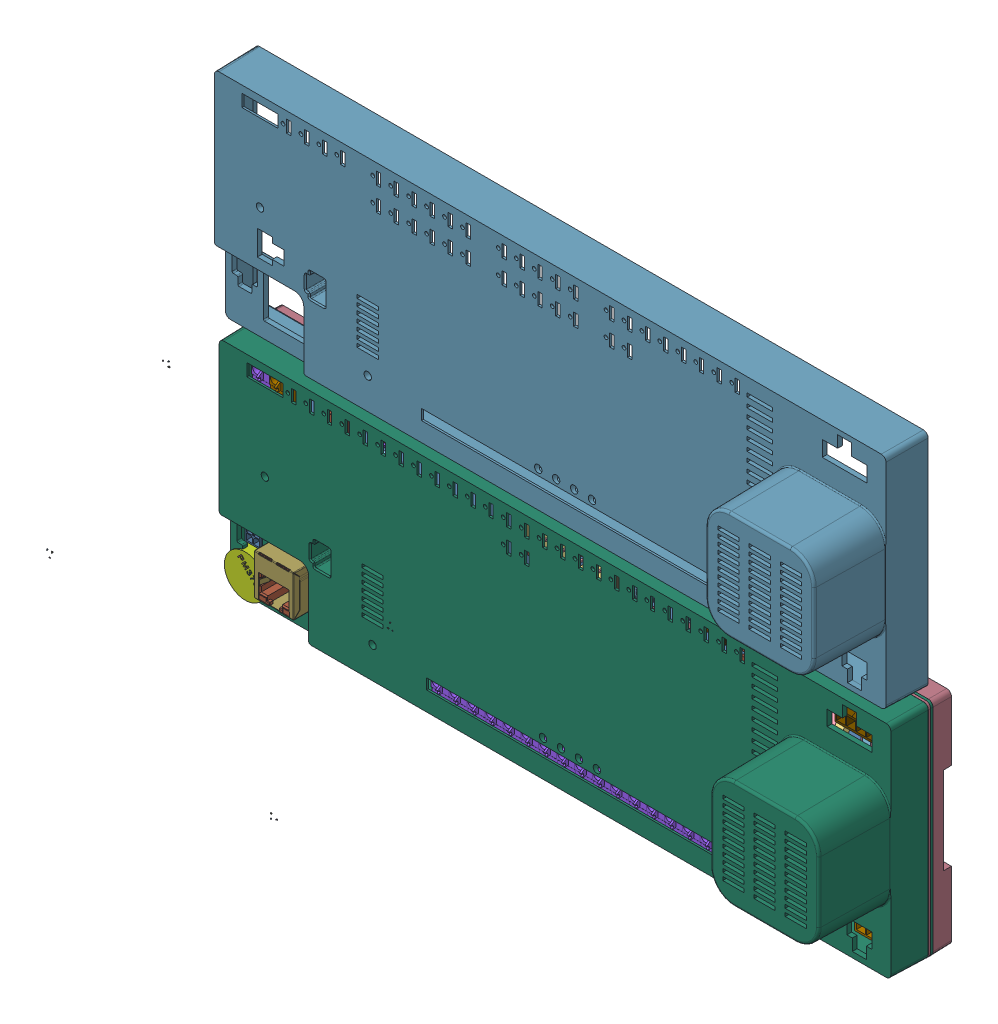
SolidWorks assembly _SC944D, configuration Default. Lengths in mm. (continued)
Components (placement in the parent): (continued)
- D13-1: D13 [Default] at origin size (219.74 39.71 23.48)
  - SW3dPS-transistor_SOT233-1: SW3dPS-transistor_SOT233 [Default] at (216.8708 -36.2332 -21.9) x (0 -1 0) z (-1 0 0) size (2.9 1.1 1.6)
  - SW3dPS-transistor_SOT233_1-1: SW3dPS-transistor_SOT233_1 [Default] at (0.2169 -0.0362 -0.0219) x (0 -1 0) z (-1 0 0) size (2.18 2.18 2.18)
  - SW3dPS-transistor_SOT233_2-1: SW3dPS-transistor_SOT233_2 [Default] at (0.0002 0 0) x (0 -1 0) z (-1 0 0) size (2.18 2.18 2.18)
  - SW3dPS-transistor_SOT233_3-1: SW3dPS-transistor_SOT233_3 [Default] x (0 -1 0) z (-1 0 0) size (2.18 2.18 2.18)
- D14-1: D14 [Default] at origin size (58.99 94.51 23.48)
  - SW3dPS-transistor_SOT233-1: SW3dPS-transistor_SOT233 [Default] at (56.1157 91.0337 -21.9) x (0 1 0) z (1 0 0) size (2.9 1.1 1.6)
  - SW3dPS-transistor_SOT233_1-1: SW3dPS-transistor_SOT233_1 [Default] at (0.0561 0.091 -0.0219) x (0 1 0) z (1 0 0) size (2.18 2.18 2.18)
  - SW3dPS-transistor_SOT233_2-1: SW3dPS-transistor_SOT233_2 [Default] at (0.0001 0.0001 0) x (0 1 0) z (1 0 0) size (2.18 2.18 2.18)
  - SW3dPS-transistor_SOT233_3-1: SW3dPS-transistor_SOT233_3 [Default] x (0 1 0) z (1 0 0) size (2.18 2.18 2.18)
- D15-1: D15 [Default] at origin size (208.53 39.58 23.48)
  - SW3dPS-transistor_SOT233-1: SW3dPS-transistor_SOT233 [Default] at (205.6631 -36.1062 -21.9) x (0 -1 0) z (-1 0 0) size (2.9 1.1 1.6)
  - SW3dPS-transistor_SOT233_1-1: SW3dPS-transistor_SOT233_1 [Default] at (0.2057 -0.0361 -0.0219) x (0 -1 0) z (-1 0 0) size (2.18 2.18 2.18)
  - SW3dPS-transistor_SOT233_2-1: SW3dPS-transistor_SOT233_2 [Default] at (0.0002 0 0) x (0 -1 0) z (-1 0 0) size (2.18 2.18 2.18)
  - SW3dPS-transistor_SOT233_3-1: SW3dPS-transistor_SOT233_3 [Default] x (0 -1 0) z (-1 0 0) size (2.18 2.18 2.18)
- D16-1: D16 [Default] at origin size (203.36 8.66 23.48)
  - SW3dPS-transistor_SOT233-1: SW3dPS-transistor_SOT233 [Default] at (200.4878 5.1688 -21.9) x (0 -1 0) z (-1 0 0) size (2.9 1.1 1.6)
  - SW3dPS-transistor_SOT233_1-1: SW3dPS-transistor_SOT233_1 [Default] at (0.2005 0.0052 -0.0219) x (0 -1 0) z (-1 0 0) size (2.18 2.18 2.18)
  - SW3dPS-transistor_SOT233_2-1: SW3dPS-transistor_SOT233_2 [Default] at (0.0002 0 0) x (0 -1 0) z (-1 0 0) size (2.18 2.18 2.18)
  - SW3dPS-transistor_SOT233_3-1: SW3dPS-transistor_SOT233_3 [Default] x (0 -1 0) z (-1 0 0) size (2.18 2.18 2.18)
- D17-1: D17 [Default] at origin size (2.6 5.2 2.43)
  - SW3dPS-DO-214AC_SMA-1: SW3dPS-DO-214AC_SMA [Default] at (158.496 76.835 1.3) x (-1 0 0) z (0 0 1) size (2.6 5.2 2.43)
- D18-1: D18 [Default] at origin size (189.01 5.29 23.48)
  - SW3dPS-transistor_SOT233-1: SW3dPS-transistor_SOT233 [Default] at (186.1368 -1.8162 -21.9) x (0 -1 0) z (-1 0 0) size (2.9 1.1 1.6)
  - SW3dPS-transistor_SOT233_1-1: SW3dPS-transistor_SOT233_1 [Default] at (0.1861 -0.0018 -0.0219) x (0 -1 0) z (-1 0 0) size (2.18 2.18 2.18)
  - SW3dPS-transistor_SOT233_2-1: SW3dPS-transistor_SOT233_2 [Default] at (0.0002 0 0) x (0 -1 0) z (-1 0 0) size (2.18 2.18 2.18)
  - SW3dPS-transistor_SOT233_3-1: SW3dPS-transistor_SOT233_3 [Default] x (0 -1 0) z (-1 0 0) size (2.18 2.18 2.18)
- D19-1: D19 [Default] at origin size (2.6 5.2 2.43)
  - SW3dPS-DO-214AC_SMA-1: SW3dPS-DO-214AC_SMA [Default] at (173.99 66.929 1.3) x (1 0 0) z (0 0 1) size (2.6 5.2 2.43)
- D20-1: D20 [Default] at origin size (5.2 2.6 2.43)
  - SW3dPS-DO-214AC_SMA-1: SW3dPS-DO-214AC_SMA [Default] at (172.339 72.136 1.3) x (0 -1 0) z (0 0 1) size (2.6 5.2 2.43)
- D24-1: D24 [Default] at origin size (119.38 129.94 23.48)
  - SW3dPS-transistor_SOT233-1: SW3dPS-transistor_SOT233 [Default] at (116.5042 126.4591 -21.9) x (0 1 0) z (1 0 0) size (2.9 1.1 1.6)
  - SW3dPS-transistor_SOT233_1-1: SW3dPS-transistor_SOT233_1 [Default] at (0.1165 0.1265 -0.0219) x (0 1 0) z (1 0 0) size (2.18 2.18 2.18)
  - SW3dPS-transistor_SOT233_2-1: SW3dPS-transistor_SOT233_2 [Default] at (0.0001 0.0001 0) x (0 1 0) z (1 0 0) size (2.18 2.18 2.18)
  - SW3dPS-transistor_SOT233_3-1: SW3dPS-transistor_SOT233_3 [Default] x (0 1 0) z (1 0 0) size (2.18 2.18 2.18)
- D26-1: D26 [Default] at origin size (119.93 45.46 23.48)
  - SW3dPS-transistor_SOT233-1: SW3dPS-transistor_SOT233 [Default] at (116.5478 42.5902 -21.9) x (-1 0 0) z (0 1 0) size (2.9 1.1 1.6)
  - SW3dPS-transistor_SOT233_1-1: SW3dPS-transistor_SOT233_1 [Default] at (0.1165 0.0426 -0.0219) x (-1 0 0) z (0 1 0) size (2.18 2.18 2.18)
  - SW3dPS-transistor_SOT233_2-1: SW3dPS-transistor_SOT233_2 [Default] at (0.0001 0 0) x (-1 0 0) z (0 1 0) size (2.18 2.18 2.18)
  - SW3dPS-transistor_SOT233_3-1: SW3dPS-transistor_SOT233_3 [Default] x (-1 0 0) z (0 1 0) size (2.18 2.18 2.18)
- D27-1: D27 [Default] at origin size (5.2 2.6 2.43)
  - SW3dPS-DO-214AC_SMA-1: SW3dPS-DO-214AC_SMA [Default] at (38.735 48.4187 1.3) x (0 1 0) z (0 0 1) size (2.6 5.2 2.43)
- D30-1: D30 [Default] at origin size (198.37 145.47 23.48)
  - SW3dPS-transistor_SOT233-1: SW3dPS-transistor_SOT233 [Default] at (195.4982 141.9924 -21.9) x (0 1 0) z (1 0 0) size (2.9 1.1 1.6)
  - SW3dPS-transistor_SOT233_1-1: SW3dPS-transistor_SOT233_1 [Default] at (0.1955 0.142 -0.0219) x (0 1 0) z (1 0 0) size (2.18 2.18 2.18)
  - SW3dPS-transistor_SOT233_2-1: SW3dPS-transistor_SOT233_2 [Default] at (0.0002 0.0001 0) x (0 1 0) z (1 0 0) size (2.18 2.18 2.18)
  - SW3dPS-transistor_SOT233_3-1: SW3dPS-transistor_SOT233_3 [Default] x (0 1 0) z (1 0 0) size (2.18 2.18 2.18)
- D33-1: D33 [Default] at origin size (1.9 2.9 0.99)
  - 1175072624-1: 1175072624 [Default] at (7.747 13.081 0) size (1.9 2.9 0.98)
    - Extruded_17-1: Extruded_17 [Default] at origin size (1.9 2.9 0.98)
  - 1175072488-1: 1175072488 [Default] at (7.747 13.716 0.95) size (1.78 0.25 0.04)
    - Extruded_18-1: Extruded_18 [Default] at origin size (1.78 0.25 0.04)
- D34-1: D34 [Default] at origin size (1.9 2.9 0.99)
  - 1175072624-1: 1175072624 [Default] at (-2.54 20.701 0) size (1.9 2.9 0.98)
    - Extruded_17-1: Extruded_17 [Default] at origin size (1.9 2.9 0.98)
  - 1175072488-1: 1175072488 [Default] at (-2.54 20.066 0.95) size (1.78 0.25 0.04)
    - Extruded_18-1: Extruded_18 [Default] at origin size (1.78 0.25 0.04)
- D43-1: D43 [Default] at origin size (168.91 55.37 23.48)
  - SW3dPS-transistor_SOT233-1: SW3dPS-transistor_SOT233 [Default] at (165.5698 52.4962 -21.9) x (-1 0 0) z (0 1 0) size (2.9 1.1 1.6)
  - SW3dPS-transistor_SOT233_1-1: SW3dPS-transistor_SOT233_1 [Default] at (0.1656 0.0525 -0.0219) x (-1 0 0) z (0 1 0) size (2.18 2.18 2.18)
  - SW3dPS-transistor_SOT233_2-1: SW3dPS-transistor_SOT233_2 [Default] at (0.0002 0.0001 0) x (-1 0 0) z (0 1 0) size (2.18 2.18 2.18)
  - SW3dPS-transistor_SOT233_3-1: SW3dPS-transistor_SOT233_3 [Default] x (-1 0 0) z (0 1 0) size (2.18 2.18 2.18)
- D46-1: D46 [Default] at origin size (232.03 39.74 23.48)
  - SW3dPS-transistor_SOT233-1: SW3dPS-transistor_SOT233 [Default] at (229.1581 -36.2649 -21.9) x (0 -1 0) z (-1 0 0) size (2.9 1.1 1.6)
  - SW3dPS-transistor_SOT233_1-1: SW3dPS-transistor_SOT233_1 [Default] at (0.2292 -0.0363 -0.0219) x (0 -1 0) z (-1 0 0) size (2.18 2.18 2.18)
  - SW3dPS-transistor_SOT233_2-1: SW3dPS-transistor_SOT233_2 [Default] at (0.0002 0 0) x (0 -1 0) z (-1 0 0) size (2.18 2.18 2.18)
  - SW3dPS-transistor_SOT233_3-1: SW3dPS-transistor_SOT233_3 [Default] x (0 -1 0) z (-1 0 0) size (2.18 2.18 2.18)
- D48-1: D48 [Default] at origin size (173.57 50.58 23.48)
  - SW3dPS-transistor_SOT233-1: SW3dPS-transistor_SOT233 [Default] at (170.0912 47.7068 -21.9) x (1 0 0) z (0 -1 0) size (2.9 1.1 1.6)
  - SW3dPS-transistor_SOT233_1-1: SW3dPS-transistor_SOT233_1 [Default] at (0.1701 0.0477 -0.0219) x (1 0 0) z (0 -1 0) size (2.18 2.18 2.18)
  - SW3dPS-transistor_SOT233_2-1: SW3dPS-transistor_SOT233_2 [Default] at (0.0002 0 0) x (1 0 0) z (0 -1 0) size (2.18 2.18 2.18)
  - SW3dPS-transistor_SOT233_3-1: SW3dPS-transistor_SOT233_3 [Default] x (1 0 0) z (0 -1 0) size (2.18 2.18 2.18)
- D49-1: D49 [Default] at origin size (64.03 38.19 23.48)
  - SW3dPS-transistor_SOT233-1: SW3dPS-transistor_SOT233 [Default] at (-60.5537 35.3194 -21.9) x (-1 0 0) z (0 1 0) size (2.9 1.1 1.6)
  - SW3dPS-transistor_SOT233_1-1: SW3dPS-transistor_SOT233_1 [Default] at (-0.0606 0.0353 -0.0219) x (-1 0 0) z (0 1 0) size (2.18 2.18 2.18)
  - SW3dPS-transistor_SOT233_2-1: SW3dPS-transistor_SOT233_2 [Default] at (-0.0001 0 0) x (-1 0 0) z (0 1 0) size (2.18 2.18 2.18)
  - SW3dPS-transistor_SOT233_3-1: SW3dPS-transistor_SOT233_3 [Default] x (-1 0 0) z (0 1 0) size (2.18 2.18 2.18)
- D50-1: D50 [Default] at origin size (181.1 140.17 23.48)
  - SW3dPS-transistor_SOT233-1: SW3dPS-transistor_SOT233 [Default] at (178.2262 136.6902 -21.9) x (0 1 0) z (1 0 0) size (2.9 1.1 1.6)
  - SW3dPS-transistor_SOT233_1-1: SW3dPS-transistor_SOT233_1 [Default] at (0.1782 0.1367 -0.0219) x (0 1 0) z (1 0 0) size (2.18 2.18 2.18)
  - SW3dPS-transistor_SOT233_2-1: SW3dPS-transistor_SOT233_2 [Default] at (0.0002 0.0001 0) x (0 1 0) z (1 0 0) size (2.18 2.18 2.18)
  - SW3dPS-transistor_SOT233_3-1: SW3dPS-transistor_SOT233_3 [Default] x (0 1 0) z (1 0 0) size (2.18 2.18 2.18)
- D51-1: D51 [Default] at origin size (15.65 146.26 23.48)
  - SW3dPS-transistor_SOT233-1: SW3dPS-transistor_SOT233 [Default] at (-12.7818 142.7862 -21.9) x (0 1 0) z (1 0 0) size (2.9 1.1 1.6)
  - SW3dPS-transistor_SOT233_1-1: SW3dPS-transistor_SOT233_1 [Default] at (-0.0128 0.1428 -0.0219) x (0 1 0) z (1 0 0) size (2.18 2.18 2.18)
  - SW3dPS-transistor_SOT233_2-1: SW3dPS-transistor_SOT233_2 [Default] at (0 0.0001 0) x (0 1 0) z (1 0 0) size (2.18 2.18 2.18)
  - SW3dPS-transistor_SOT233_3-1: SW3dPS-transistor_SOT233_3 [Default] x (0 1 0) z (1 0 0) size (2.18 2.18 2.18)
- D53-1: D53 [Default] at origin size (2.6 1.36 1.13)
  - SW3dPS-SOD-323-1: SW3dPS-SOD-323 [Default] at (48.4186 68.7386 0) x (-1 0 0) z (0 0 1) size (2.6 1.36 1.13)
- D54-1: D54 [Default] at origin size (133.48 48.35 23.48)
  - SW3dPS-transistor_SOT233-1: SW3dPS-transistor_SOT233 [Default] at (130.1051 45.4794 -21.9) x (-1 0 0) z (0 1 0) size (2.9 1.1 1.6)
  - SW3dPS-transistor_SOT233_1-1: SW3dPS-transistor_SOT233_1 [Default] at (0.1301 0.0455 -0.0219) x (-1 0 0) z (0 1 0) size (2.18 2.18 2.18)
  - SW3dPS-transistor_SOT233_2-1: SW3dPS-transistor_SOT233_2 [Default] at (0.0001 0 0) x (-1 0 0) z (0 1 0) size (2.18 2.18 2.18)
  - SW3dPS-transistor_SOT233_3-1: SW3dPS-transistor_SOT233_3 [Default] x (-1 0 0) z (0 1 0) size (2.18 2.18 2.18)
- D56-1: D56 [Default] at origin size (230.54 11.39 23.48)
  - SW3dPS-transistor_SOT233-1: SW3dPS-transistor_SOT233 [Default] at (227.6658 -7.9122 -21.9) x (0 -1 0) z (-1 0 0) size (2.9 1.1 1.6)
  - SW3dPS-transistor_SOT233_1-1: SW3dPS-transistor_SOT233_1 [Default] at (0.2277 -0.0079 -0.0219) x (0 -1 0) z (-1 0 0) size (2.18 2.18 2.18)
  - SW3dPS-transistor_SOT233_2-1: SW3dPS-transistor_SOT233_2 [Default] at (0.0002 0 0) x (0 -1 0) z (-1 0 0) size (2.18 2.18 2.18)
  - SW3dPS-transistor_SOT233_3-1: SW3dPS-transistor_SOT233_3 [Default] x (0 -1 0) z (-1 0 0) size (2.18 2.18 2.18)
- D57-1: D57 [Default] at origin size (72.61 38.22 23.48)
  - SW3dPS-transistor_SOT233-1: SW3dPS-transistor_SOT233 [Default] at (69.1768 35.3512 -21.9) x (-1 0 0) z (0 1 0) size (2.9 1.1 1.6)
  - SW3dPS-transistor_SOT233_1-1: SW3dPS-transistor_SOT233_1 [Default] at (0.0692 0.0354 -0.0219) x (-1 0 0) z (0 1 0) size (2.18 2.18 2.18)
  - SW3dPS-transistor_SOT233_2-1: SW3dPS-transistor_SOT233_2 [Default] at (0.0001 0 0) x (-1 0 0) z (0 1 0) size (2.18 2.18 2.18)
  - SW3dPS-transistor_SOT233_3-1: SW3dPS-transistor_SOT233_3 [Default] x (-1 0 0) z (0 1 0) size (2.18 2.18 2.18)
- D58-1: D58 [Default] at origin size (132.49 30.35 23.48)
  - SW3dPS-transistor_SOT233-1: SW3dPS-transistor_SOT233 [Default] at (129.1208 27.4772 -21.9) x (-1 0 0) z (0 1 0) size (2.9 1.1 1.6)
  - SW3dPS-transistor_SOT233_1-1: SW3dPS-transistor_SOT233_1 [Default] at (0.1291 0.0275 -0.0219) x (-1 0 0) z (0 1 0) size (2.18 2.18 2.18)
  - SW3dPS-transistor_SOT233_2-1: SW3dPS-transistor_SOT233_2 [Default] at (0.0001 0 0) x (-1 0 0) z (0 1 0) size (2.18 2.18 2.18)
  - SW3dPS-transistor_SOT233_3-1: SW3dPS-transistor_SOT233_3 [Default] x (-1 0 0) z (0 1 0) size (2.18 2.18 2.18)
- D59-1: D59 [Default] at origin size (5.2 2.6 2.43)
  - SW3dPS-DO-214AC_SMA-1: SW3dPS-DO-214AC_SMA [Default] at (139.192 62.23 1.3) x (0 -1 0) z (0 0 1) size (2.6 5.2 2.43)
- D60-1: D60 [Default] at origin size (2.6 5.2 2.43)
  - SW3dPS-DO-214AC_SMA-1: SW3dPS-DO-214AC_SMA [Default] at (126.111 60.7619 1.3) x (1 0 0) z (0 0 1) size (2.6 5.2 2.43)
- D61-1: D61 [Default] at origin size (2.6 5.2 2.43)
  - SW3dPS-DO-214AC_SMA-1: SW3dPS-DO-214AC_SMA [Default] at (133.731 62.7024 1.3) x (1 0 0) z (0 0 1) size (2.6 5.2 2.43)
- D62-1: D62 [Default] at origin size (2.6 5.2 2.43)
  - SW3dPS-DO-214AC_SMA-1: SW3dPS-DO-214AC_SMA [Default] at (122.428 58.928 1.3) x (1 0 0) z (0 0 1) size (2.6 5.2 2.43)
- D63-1: D63 [Default] at origin size (2.6 5.2 2.43)
  - SW3dPS-DO-214AC_SMA-1: SW3dPS-DO-214AC_SMA [Default] at (26.4795 68.453 1.3) x (1 0 0) z (0 0 1) size (2.6 5.2 2.43)
- D64-1: D64 [Default] at origin size (49.9 40.25 23.48)
  - SW3dPS-transistor_SOT233-1: SW3dPS-transistor_SOT233 [Default] at (46.4438 37.3832 -21.9) x (-1 0 0) z (0 1 0) size (2.9 1.1 1.6)
  - SW3dPS-transistor_SOT233_1-1: SW3dPS-transistor_SOT233_1 [Default] at (0.0464 0.0374 -0.0219) x (-1 0 0) z (0 1 0) size (2.18 2.18 2.18)
  - SW3dPS-transistor_SOT233_2-1: SW3dPS-transistor_SOT233_2 [Default] at (0 0 0) x (-1 0 0) z (0 1 0) size (2.18 2.18 2.18)
  - SW3dPS-transistor_SOT233_3-1: SW3dPS-transistor_SOT233_3 [Default] x (-1 0 0) z (0 1 0) size (2.18 2.18 2.18)
- D65-1: D65 [Default] at origin size (2.6 1.36 1.13)
  - SW3dPS-SOD-323-1: SW3dPS-SOD-323 [Default] at (69.2149 51.5619 0) x (-1 0 0) z (0 0 1) size (2.6 1.36 1.13)
- DL6-1: DL6 [Default] at origin size (2.03 1.27 1.16)
  - SW3dPS-led805R-1-1: SW3dPS-led805R-1 [Default] at (12.6999 44.9201 0) x (0 1 0) z (1 0 0) size (1.27 1.11 2.03)
  - 1175072760-1: 1175072760 [Default] at (12.7 44.92 0.508) size (1.52 1.27 0.64)
    - Extruded_19-1: Extruded_19 [Default] at origin size (1.52 1.27 0.64)
- DL7-1: DL7 [Default] at origin size (2.03 1.27 1.11)
  - SW3dPS-led805-1: SW3dPS-led805 [Default] at (58.4201 5.9201 0) x (0 1 0) z (1 0 0) size (1.27 1.11 2.03)
- F1-1: F1 [Default] at origin size (10.9 3 3)
  - SW3dPS-UMT250-1: SW3dPS-UMT250 [Default] at (197.1676 9.8426 1.5) x (1 0 0) z (0 0 1) size (10.9 3 3)
- F2-1: F2 [Default] at origin size (10.9 3 3)
  - SW3dPS-UMT250-1: SW3dPS-UMT250 [Default] at (211.4551 9.8426 1.5) x (1 0 0) z (0 0 1) size (10.9 3 3)
- F3-1: F3 [Default] at origin size (19.94 11.4 8.17)
  - WE-SLM_744242_2021910280-1: WE-SLM_744242_2021910280 [Default] at (216.2175 20.9551 0) x (0 1 0) z (0.984808 0 0.173648) size (11.4 3.8 19)
    - Extruded_20-1: Extruded_20 [Default] at origin size (11.4 3.8 19)
  - 1173466816-1: 1173466816 [Default] at (216.2174 23.8551 -3) x (0 1 0) z (0 0 1) size (0.9 0.9 3)
    - Cylinder_5-1: Cylinder_5 [Default] at origin size (0.9 0.9 3)
  - 1173466816-2: 1173466816 [Default] at (216.2174 18.0551 -3) x (0 1 0) z (0 0 1) size (0.9 0.9 3)
    - Cylinder_5-1: Cylinder_5 [Default] at origin size (0.9 0.9 3)
  - 1173466688-1: 1173466688 [Default] at (216.2174 23.8551 0) x (0 1 0) z (0 0 1) size (1.8 1.8 2)
    - Cylinder_2-1: Cylinder_2 [Default] at origin size (1.8 1.8 2)
  - 1173466688-2: 1173466688 [Default] at (216.2174 18.0551 0) x (0 1 0) z (0 0 1) size (1.8 1.8 2)
    - Cylinder_2-1: Cylinder_2 [Default] at origin size (1.8 1.8 2)
- F4-1: F4 [Default] at origin size (10.9 3 3)
  - SW3dPS-UMT250-1: SW3dPS-UMT250 [Default] at (182.7213 9.8426 1.5) x (1 0 0) z (0 0 1) size (10.9 3 3)
- J1-1: J1 [Default] at origin size (9.42 10 19.2)
  - 1790377-1: 1790377 [Default] at (12.7001 72.9201 0) x (0 1 0) z (1 0 0) size (10 19.2 9.42)
    - ffkdsa-v2-7.62-1: ffkdsa-v2-7.62 [Default] at (-23.7414 -38.158 -5.08) x (0 -1 0) z (0 0 1) size (19.2 10 9.42)
- J2-1: J2 [Default] at origin size (7.62 10 19.2)
  - 1790487-1: 1790487 [Default] at (6.12 64.87 -10.6348) x (0 1 0) z (1 0 0) size (10 19.2 7.62)
    - ffkdsa1-v2-7.62-1: ffkdsa1-v2-7.62 [Default] at (-15.6914 -27.508 9.12) x (0 -1 0) z (0 0 1) size (19.2 10 7.62)
- J31-1: J31 [Default] at origin size (10 8.67 12.42)
  - c-3-794630-4-g-3d-1: c-3-794630-4-g-3d [Default] at (1.4199 14.1799 9.3) x (-1 0 0) z (0 0 1) size (10 8.67 12.42)
- J32-1: J32 [Default] at origin size (17.21 17.5 21.01)
  - 74990101210-1: 74990101210 [Default] at (18.4201 6.6501 0) size (17.21 17.5 21.01)
    - base-1: base [Default] at origin size (16.4 17.1 20.81)
    - shielding-1: shielding [Default] at origin size (17.21 17.5 21)
- J33-1: J33 [Default] at origin size (12.7 5.08 10.6)
  - 1175074800-1: 1175074800 [Default] at (49.657 49.911 0) size (12.7 5.08 2.61)
    - Extruded_4-1: Extruded_4 [Default] at origin size (12.7 5.08 2.61)
  - 1175073304-1: 1175073304 [Default] at (44.577 48.641 -2) size (0.76 0.76 2)
    - Extruded_5-1: Extruded_5 [Default] at origin size (0.76 0.76 2)
  - 1175073168-1: 1175073168 [Default] at (44.577 48.641 0) size (0.76 0.76 8.6)
    - Extruded_6-1: Extruded_6 [Default] at origin size (0.76 0.76 8.6)
  - 1175073304-2: 1175073304 [Default] at (44.577 51.181 -2) size (0.76 0.76 2)
    - Extruded_5-1: Extruded_5 [Default] at origin size (0.76 0.76 2)
  - 1175073168-2: 1175073168 [Default] at (44.577 51.181 0) size (0.76 0.76 8.6)
    - Extruded_6-1: Extruded_6 [Default] at origin size (0.76 0.76 8.6)
  - 1175073304-3: 1175073304 [Default] at (47.117 51.181 -2) size (0.76 0.76 2)
    - Extruded_5-1: Extruded_5 [Default] at origin size (0.76 0.76 2)
  - 1175073168-3: 1175073168 [Default] at (47.117 51.181 0) size (0.76 0.76 8.6)
    - Extruded_6-1: Extruded_6 [Default] at origin size (0.76 0.76 8.6)
  - 1175073304-4: 1175073304 [Default] at (47.117 48.641 -2) size (0.76 0.76 2)
    - Extruded_5-1: Extruded_5 [Default] at origin size (0.76 0.76 2)
  - 1175073168-4: 1175073168 [Default] at (47.117 48.641 0) size (0.76 0.76 8.6)
    - Extruded_6-1: Extruded_6 [Default] at origin size (0.76 0.76 8.6)
  - 1175073304-5: 1175073304 [Default] at (49.657 48.641 -2) size (0.76 0.76 2)
    - Extruded_5-1: Extruded_5 [Default] at origin size (0.76 0.76 2)
  - 1175073168-5: 1175073168 [Default] at (49.657 48.641 0) size (0.76 0.76 8.6)
    - Extruded_6-1: Extruded_6 [Default] at origin size (0.76 0.76 8.6)
  - 1175073304-6: 1175073304 [Default] at (49.657 51.181 -2) size (0.76 0.76 2)
    - Extruded_5-1: Extruded_5 [Default] at origin size (0.76 0.76 2)
  - 1175073168-6: 1175073168 [Default] at (49.657 51.181 0) size (0.76 0.76 8.6)
    - Extruded_6-1: Extruded_6 [Default] at origin size (0.76 0.76 8.6)
  - 1175073304-7: 1175073304 [Default] at (52.197 51.181 -2) size (0.76 0.76 2)
    - Extruded_5-1: Extruded_5 [Default] at origin size (0.76 0.76 2)
  - 1175073168-7: 1175073168 [Default] at (52.197 51.181 0) size (0.76 0.76 8.6)
    - Extruded_6-1: Extruded_6 [Default] at origin size (0.76 0.76 8.6)
  - 1175073304-8: 1175073304 [Default] at (52.197 48.641 -2) size (0.76 0.76 2)
    - Extruded_5-1: Extruded_5 [Default] at origin size (0.76 0.76 2)
  - 1175073168-8: 1175073168 [Default] at (52.197 48.641 0) size (0.76 0.76 8.6)
    - Extruded_6-1: Extruded_6 [Default] at origin size (0.76 0.76 8.6)
  - 1175073304-9: 1175073304 [Default] at (54.737 48.641 -2) size (0.76 0.76 2)
    - Extruded_5-1: Extruded_5 [Default] at origin size (0.76 0.76 2)
  - 1175073168-9: 1175073168 [Default] at (54.737 48.641 0) size (0.76 0.76 8.6)
    - Extruded_6-1: Extruded_6 [Default] at origin size (0.76 0.76 8.6)
  - 1175073304-10: 1175073304 [Default] at (54.737 51.181 -2) size (0.76 0.76 2)
    - Extruded_5-1: Extruded_5 [Default] at origin size (0.76 0.76 2)
  - 1175073168-10: 1175073168 [Default] at (54.737 51.181 0) size (0.76 0.76 8.6)
    - Extruded_6-1: Extruded_6 [Default] at origin size (0.76 0.76 8.6)
- J34-1: J34 [Default] at origin size (9.42 10 19.2)
  - 1790377-1: 1790377 [Default] at (88.9 -4.0799 0) x (0 1 0) z (1 0 0) size (10 19.2 9.42)
    - ffkdsa-v2-7.62-1: ffkdsa-v2-7.62 [Default] at (-23.7414 -38.158 -5.08) x (0 -1 0) z (0 0 1) size (19.2 10 9.42)
- J35-1: J35 [Default] at origin size (9.42 10 19.2)
  - 1790377-1: 1790377 [Default] at (96.5201 -4.0799 0) x (0 1 0) z (1 0 0) size (10 19.2 9.42)
    - ffkdsa-v2-7.62-1: ffkdsa-v2-7.62 [Default] at (-23.7414 -38.158 -5.08) x (0 -1 0) z (0 0 1) size (19.2 10 9.42)
- J36-1: J36 [Default] at origin size (9.42 10 19.2)
  - 1790377-1: 1790377 [Default] at (104.1401 -4.0799 0) x (0 1 0) z (1 0 0) size (10 19.2 9.42)
    - ffkdsa-v2-7.62-1: ffkdsa-v2-7.62 [Default] at (-23.7414 -38.158 -5.08) x (0 -1 0) z (0 0 1) size (19.2 10 9.42)
- J37-1: J37 [Default] at origin size (9.42 10 19.2)
  - 1790377-1: 1790377 [Default] at (111.76 -4.0799 0) x (0 1 0) z (1 0 0) size (10 19.2 9.42)
    - ffkdsa-v2-7.62-1: ffkdsa-v2-7.62 [Default] at (-23.7414 -38.158 -5.08) x (0 -1 0) z (0 0 1) size (19.2 10 9.42)
- J38-1: J38 [Default] at origin size (9.42 10 19.2)
  - 1790377-1: 1790377 [Default] at (119.3801 -4.0799 0) x (0 1 0) z (1 0 0) size (10 19.2 9.42)
    - ffkdsa-v2-7.62-1: ffkdsa-v2-7.62 [Default] at (-23.7414 -38.158 -5.08) x (0 -1 0) z (0 0 1) size (19.2 10 9.42)
- J39-1: J39 [Default] at origin size (9.42 10 19.2)
  - 1790377-1: 1790377 [Default] at (127.0001 -4.0799 0) x (0 1 0) z (1 0 0) size (10 19.2 9.42)
    - ffkdsa-v2-7.62-1: ffkdsa-v2-7.62 [Default] at (-23.7414 -38.158 -5.08) x (0 -1 0) z (0 0 1) size (19.2 10 9.42)
- J40-1: J40 [Default] at origin size (9.42 10 19.2)
  - 1790377-1: 1790377 [Default] at (134.62 -4.0799 0) x (0 1 0) z (1 0 0) size (10 19.2 9.42)
    - ffkdsa-v2-7.62-1: ffkdsa-v2-7.62 [Default] at (-23.7414 -38.158 -5.08) x (0 -1 0) z (0 0 1) size (19.2 10 9.42)
- J41-1: J41 [Default] at origin size (9.42 10 19.2)
  - 1790377-1: 1790377 [Default] at (142.2401 -4.0799 0) x (0 1 0) z (1 0 0) size (10 19.2 9.42)
    - ffkdsa-v2-7.62-1: ffkdsa-v2-7.62 [Default] at (-23.7414 -38.158 -5.08) x (0 -1 0) z (0 0 1) size (19.2 10 9.42)
- J42-1: J42 [Default] at origin size (9.42 10 19.2)
  - 1790377-1: 1790377 [Default] at (149.8601 -4.0799 0) x (0 1 0) z (1 0 0) size (10 19.2 9.42)
    - ffkdsa-v2-7.62-1: ffkdsa-v2-7.62 [Default] at (-23.7414 -38.158 -5.08) x (0 -1 0) z (0 0 1) size (19.2 10 9.42)
- J43-1: J43 [Default] at origin size (9.42 10 19.2)
  - 1790377-1: 1790377 [Default] at (157.48 -4.0799 0) x (0 1 0) z (1 0 0) size (10 19.2 9.42)
    - ffkdsa-v2-7.62-1: ffkdsa-v2-7.62 [Default] at (-23.7414 -38.158 -5.08) x (0 -1 0) z (0 0 1) size (19.2 10 9.42)
- J44-1: J44 [Default] at origin size (9.42 10 19.2)
  - 1790377-1: 1790377 [Default] at (165.1001 -4.0799 0) x (0 1 0) z (1 0 0) size (10 19.2 9.42)
    - ffkdsa-v2-7.62-1: ffkdsa-v2-7.62 [Default] at (-23.7414 -38.158 -5.08) x (0 -1 0) z (0 0 1) size (19.2 10 9.42)
- J45-1: J45 [Default] at origin size (9.42 10 19.2)
  - 1790377-1: 1790377 [Default] at (172.7201 -4.0799 0) x (0 1 0) z (1 0 0) size (10 19.2 9.42)
    - ffkdsa-v2-7.62-1: ffkdsa-v2-7.62 [Default] at (-23.7414 -38.158 -5.08) x (0 -1 0) z (0 0 1) size (19.2 10 9.42)
- J46-1: J46 [Default] at origin size (9.42 10 19.2)
  - 1790377-1: 1790377 [Default] at (180.34 -4.0799 0) x (0 1 0) z (1 0 0) size (10 19.2 9.42)
    - ffkdsa-v2-7.62-1: ffkdsa-v2-7.62 [Default] at (-23.7414 -38.158 -5.08) x (0 -1 0) z (0 0 1) size (19.2 10 9.42)
- J47-1: J47 [Default] at origin size (9.42 10 19.2)
  - 1790377-1: 1790377 [Default] at (187.96 -4.0799 0) x (0 1 0) z (1 0 0) size (10 19.2 9.42)
    - ffkdsa-v2-7.62-1: ffkdsa-v2-7.62 [Default] at (-23.7414 -38.158 -5.08) x (0 -1 0) z (0 0 1) size (19.2 10 9.42)
- J48-1: J48 [Default] at origin size (9.42 10 19.2)
  - 1790377-1: 1790377 [Default] at (195.58 -4.0799 0) x (0 1 0) z (1 0 0) size (10 19.2 9.42)
    - ffkdsa-v2-7.62-1: ffkdsa-v2-7.62 [Default] at (-23.7414 -38.158 -5.08) x (0 -1 0) z (0 0 1) size (19.2 10 9.42)
- J49-1: J49 [Default] at origin size (9.42 10 19.2)
  - 1790377-1: 1790377 [Default] at (203.2001 -4.0799 0) x (0 1 0) z (1 0 0) size (10 19.2 9.42)
    - ffkdsa-v2-7.62-1: ffkdsa-v2-7.62 [Default] at (-23.7414 -38.158 -5.08) x (0 -1 0) z (0 0 1) size (19.2 10 9.42)
- J50-1: J50 [Default] at origin size (9.42 10 19.2)
  - 1790377-1: 1790377 [Default] at (210.8201 -4.0799 0) x (0 1 0) z (1 0 0) size (10 19.2 9.42)
    - ffkdsa-v2-7.62-1: ffkdsa-v2-7.62 [Default] at (-23.7414 -38.158 -5.08) x (0 -1 0) z (0 0 1) size (19.2 10 9.42)
- J51-1: J51 [Default] at origin size (7.62 10 19.2)
  - 1790487-1: 1790487 [Default] at (204.24 -12.13 -10.6348) x (0 1 0) z (1 0 0) size (10 19.2 7.62)
    - ffkdsa1-v2-7.62-1: ffkdsa1-v2-7.62 [Default] at (-15.6914 -27.508 9.12) x (0 -1 0) z (0 0 1) size (19.2 10 7.62)
- J52-1: J52 [Default] at origin size (9.6 6.9 16.3)
  - 64900211122-1: 64900211122 [Default] at (265.1199 3.0931 6.4152) x (-1 0 0) z (0 0 1) size (9.6 6.9 16.3)
    - 64900211122-1: 64900211122 [Default] at origin size (9.6 6.9 12.8)
    - 6490xx11122_PIN_1-1: 6490xx11122_PIN_1 [Default] at (-2.1 -0.025 -2.45) x (-1 0 0) z (0 0 -1) size (1.1 1.85 12.85)
    - 6490xx11122_PIN_1-2: 6490xx11122_PIN_1 [Default] at (2.1 -0.025 -2.45) x (-1 0 0) z (0 0 -1) size (1.1 1.85 12.85)
- J54-1: J54 [Default] at origin size (2.79 5.33 10.6)
  - 1175073304-1: 1175073304 [Default] at (46.22 29.42 -2) size (0.76 0.76 2)
    - Extruded_5-1: Extruded_5 [Default] at origin size (0.76 0.76 2)
  - 1175073440-1: 1175073440 [Default] at (46.22 30.69 0) size (2.79 5.33 2.6)
    - Extruded_7-1: Extruded_7 [Default] at origin size (2.79 5.33 2.6)
  - 1175073168-1: 1175073168 [Default] at (46.22 29.42 0) size (0.76 0.76 8.6)
    - Extruded_6-1: Extruded_6 [Default] at origin size (0.76 0.76 8.6)
  - 1175073168-2: 1175073168 [Default] at (46.22 31.96 0) size (0.76 0.76 8.6)
    - Extruded_6-1: Extruded_6 [Default] at origin size (0.76 0.76 8.6)
  - 1175073304-2: 1175073304 [Default] at (46.22 31.96 -2) size (0.76 0.76 2)
    - Extruded_5-1: Extruded_5 [Default] at origin size (0.76 0.76 2)
- J56-1: J56 [Default] at origin size (18 6.9 16.3)
  - 64900411122-1: 64900411122 [Default] at (260.9201 75.8104 6.4152) x (1 0 0) z (0 0 1) size (18 6.9 16.3)
    - 6490xx11122_PIN-1: 6490xx11122_PIN [Default] at (-6.3 -0.025 -2.45) x (-1 0 0) z (0 0 -1) size (1.1 1.85 12.85)
    - 6490xx11122_PIN-2: 6490xx11122_PIN [Default] at (-2.1 -0.025 -2.45) x (-1 0 0) z (0 0 -1) size (1.1 1.85 12.85)
    - 6490xx11122_PIN-3: 6490xx11122_PIN [Default] at (2.1 -0.025 -2.45) x (-1 0 0) z (0 0 -1) size (1.1 1.85 12.85)
    - 6490xx11122_PIN-4: 6490xx11122_PIN [Default] at (6.3 -0.025 -2.45) x (-1 0 0) z (0 0 -1) size (1.1 1.85 12.85)
    - 64900411122-1: 64900411122 [Default] at origin size (18 6.9 12.8)
- J58-1: J58 [Default] at origin size (2.79 5.33 10.6)
  - 1175073304-1: 1175073304 [Default] at (36.92 28.194 -2) size (0.76 0.76 2)
    - Extruded_5-1: Extruded_5 [Default] at origin size (0.76 0.76 2)
  - 1175073440-1: 1175073440 [Default] at (36.92 26.924 0) size (2.79 5.33 2.6)
    - Extruded_7-1: Extruded_7 [Default] at origin size (2.79 5.33 2.6)
  - 1175073168-1: 1175073168 [Default] at (36.92 28.194 0) size (0.76 0.76 8.6)
    - Extruded_6-1: Extruded_6 [Default] at origin size (0.76 0.76 8.6)
  - 1175073168-2: 1175073168 [Default] at (36.92 25.654 0) size (0.76 0.76 8.6)
    - Extruded_6-1: Extruded_6 [Default] at origin size (0.76 0.76 8.6)
  - 1175073304-2: 1175073304 [Default] at (36.92 25.654 -2) size (0.76 0.76 2)
    - Extruded_5-1: Extruded_5 [Default] at origin size (0.76 0.76 2)
- J102-1: J102 [Default] at origin size (10.16 2.54 10.6)
  - 1175074936-1: 1175074936 [Default] at (54.864 -1.524 0) size (10.16 2.54 2.61)
    - Extruded_8-1: Extruded_8 [Default] at origin size (10.16 2.54 2.61)
  - 1175073304-1: 1175073304 [Default] at (51.054 -1.524 -2) size (0.76 0.76 2)
    - Extruded_5-1: Extruded_5 [Default] at origin size (0.76 0.76 2)
  - 1175073168-1: 1175073168 [Default] at (51.054 -1.524 0) size (0.76 0.76 8.6)
    - Extruded_6-1: Extruded_6 [Default] at origin size (0.76 0.76 8.6)
  - 1175073304-2: 1175073304 [Default] at (53.594 -1.524 -2) size (0.76 0.76 2)
    - Extruded_5-1: Extruded_5 [Default] at origin size (0.76 0.76 2)
  - 1175073168-2: 1175073168 [Default] at (53.594 -1.524 0) size (0.76 0.76 8.6)
    - Extruded_6-1: Extruded_6 [Default] at origin size (0.76 0.76 8.6)
  - 1175073304-3: 1175073304 [Default] at (56.134 -1.524 -2) size (0.76 0.76 2)
    - Extruded_5-1: Extruded_5 [Default] at origin size (0.76 0.76 2)
  - 1175073168-3: 1175073168 [Default] at (56.134 -1.524 0) size (0.76 0.76 8.6)
    - Extruded_6-1: Extruded_6 [Default] at origin size (0.76 0.76 8.6)
  - 1175073304-4: 1175073304 [Default] at (58.674 -1.524 -2) size (0.76 0.76 2)
    - Extruded_5-1: Extruded_5 [Default] at origin size (0.76 0.76 2)
  - 1175073168-4: 1175073168 [Default] at (58.674 -1.524 0) size (0.76 0.76 8.6)
    - Extruded_6-1: Extruded_6 [Default] at origin size (0.76 0.76 8.6)
- K1-1: K1 [Default] at origin size (11 21 10.7)
  - 1175073576-1: 1175073576 [Default] at (196.683 23.779 0) size (11 21 10.7)
    - Extruded_9-1: Extruded_9 [Default] at origin size (11 21 10.7)
- K2-1: K2 [Default] at origin size (11 21 10.7)
  - 1175073576-1: 1175073576 [Default] at (208.375 23.779 0) size (11 21 10.7)
    - Extruded_9-1: Extruded_9 [Default] at origin size (11 21 10.7)
- K3-1: K3 [Default] at origin size (21 11 10.7)
  - 1175073712-1: 1175073712 [Default] at (91.8863 16.6687 0) size (21 11 10.7)
    - Extruded_10-1: Extruded_10 [Default] at origin size (21 11 10.7)
- K5-1: K5 [Default] at origin size (11 21 10.7)
  - 1175073576-1: 1175073576 [Default] at (185.118 23.779 0) size (11 21 10.7)
    - Extruded_9-1: Extruded_9 [Default] at origin size (11 21 10.7)
- L1-1: L1 [Default] at origin size (4.5 3.2 2.3)
  - WE-MPSB_1812_MPSB-1: WE-MPSB_1812_MPSB [Default] at (254.8891 61.722 1.1652) x (0 -1 0) z (0 0 1) size (3.2 4.5 2.3)
    - Base_1-1: Base_1 [Default] at (0 -1.79 0) size (3.2 0.46 2.3)
    - Base_1-2: Base_1 [Default] at (0 1.79 0) x (-1 0 0) z (0 0 1) size (3.2 0.46 2.3)
    - Ferrite-1: Ferrite [Default] at origin size (3.2 3.58 2.3)
- L2-1: L2 [Default] at origin size (6 9.2 5)
  - WE-SL2_74422-1: WE-SL2_74422 [Default] at (31.8134 66.675 0) x (0 1 0) z (0 0 1) size (9.2 6 5)
    - Boden-1: Boden [Default] at origin size (1.75 1 3.2)
    - Boden_1-1: Boden_1 [Default] at origin size (1.75 1 3.2)
    - Boden_2-1: Boden_2 [Default] at origin size (9.2 6 2.8)
    - Boden_3-1: Boden_3 [Default] at origin size (1.75 1 3.2)
    - Boden_4-1: Boden_4 [Default] at origin size (1.75 1 3.2)
    - Deckel-1: Deckel [Default] at (0 0 2) size (9.2 6 3)
- L3-1: L3 [Default] at origin size (1.6 3.2 1)
  - SW3dPS-1206_SMD_Resistor-1: SW3dPS-1206_SMD_Resistor [Default] at (79.502 52.906 0) x (0 -1 0) z (-1 0 0) size (3.2 1 1.6)
- L4-1: L4 [Default] at origin size (1.6 0.8 0.9)
  - User_Library-CAPC1608X09-1: User_Library-CAPC1608X09 [Default] at (40.6401 70.9613 0) x (1 0 0) z (0 0 1) size (1.6 0.8 0.9)
- L5-1: L5 [Default] at origin size (1.6 0.8 0.9)
  - User_Library-CAPC1608X09-1: User_Library-CAPC1608X09 [Default] at (55.5307 81.3752 0) x (-1 0 0) z (0 0 1) size (1.6 0.8 0.9)
- L6-1: L6 [Default] at origin size (3.3 6 3.25)
  - WE-SLM_744242_2286829984-1: WE-SLM_744242_2286829984 [Default] at (158.6229 69.0879 1.7653) x (1 0 0) z (0 0 -1) size (2.82 6 3)
  - WE-SLM_744242_2286829984_1-1: WE-SLM_744242_2286829984_1 [Default] at (158.6229 69.0879 1.7653) x (1 0 0) z (0 0 -1) size (3.3 5 3)
- L7-1: L7 [Default] at origin size (6 3.3 3.25)
  - WE-SLM_744242_2286829984-1: WE-SLM_744242_2286829984 [Default] at (180.3401 70.4849 1.7653) x (0 1 0) z (0 0 -1) size (2.82 6 3)
  - WE-SLM_744242_2286829984_1-1: WE-SLM_744242_2286829984_1 [Default] at (180.3401 70.4849 1.7653) x (0 1 0) z (0 0 -1) size (3.3 5 3)
- L8-1: L8 [Default] at origin size (1.6 0.8 0.9)
  - User_Library-CAPC1608X09-1: User_Library-CAPC1608X09 [Default] at (56.0388 70.4851 0) x (1 0 0) z (0 0 1) size (1.6 0.8 0.9)
- L9-1: L9 [Default] at origin size (1.6 0.8 0.9)
  - User_Library-CAPC1608X09-1: User_Library-CAPC1608X09 [Default] at (100.5839 78.7399 0) x (-1 0 0) z (0 0 1) size (1.6 0.8 0.9)
- L10-1: L10 [Default] at origin size (12 12 10.38)
  - WE-PD_1210_Metal_TYPE_XXL_12x12xh10-1: WE-PD_1210_Metal_TYPE_XXL_12x12xh10 [Default] at (228.2825 60.4837 5.2652) x (0 1 0) z (0 0 1) size (12 12 10.38)
    - Lötfläche-1: Lötfläche [Default] at (0 0 -5.25) x (0 1 0) z (0 0 1) size (5 9.29 3.02)
    - Lötfläche_1-1: Lötfläche_1 [Default] at (0 0 -5.25) x (0 1 0) z (0 0 1) size (5 9.29 3.02)
    - 7447709001-1: 7447709001 [Default] at origin size (9.09 9.09 6.26)
    - 7447709001_1-1: 7447709001_1 [Default] at origin size (12 12 10.13)
    - 7447709001_2-1: 7447709001_2 [Default] at origin size (6.34 6.34 6.57)
- L11-1: L11 [Default] at origin size (4.5 3.2 2.3)
  - WE-MPSB_1812_MPSB-1: WE-MPSB_1812_MPSB [Default] at (225.5837 35.0838 1.1652) x (0 1 0) z (0 0 1) size (3.2 4.5 2.3)
    - Base_1-1: Base_1 [Default] at (0 -1.79 0) size (3.2 0.46 2.3)
    - Base_1-2: Base_1 [Default] at (0 1.79 0) x (-1 0 0) z (0 0 1) size (3.2 0.46 2.3)
    - Ferrite-1: Ferrite [Default] at origin size (3.2 3.58 2.3)
- L12-1: L12 [Default] at origin size (1.6 0.8 0.9)
  - User_Library-CAPC1608X09-1: User_Library-CAPC1608X09 [Default] at (181.9269 51.9429 0) x (-1 0 0) z (0 0 1) size (1.6 0.8 0.9)
- L13-1: L13 [Default] at origin size (1.6 3.2 1)
  - SW3dPS-1206_SMD_Resistor-1: SW3dPS-1206_SMD_Resistor [Default] at (68.072 56.843 0) x (0 -1 0) z (-1 0 0) size (3.2 1 1.6)
- L14-1: L14 [Default] at origin size (4.8 4.8 2.8)
  - WE-TPC_4828-1: WE-TPC_4828 [Default] at (68.8341 47.498 2.794) x (0 -1 0) z (0 0 1) size (4.8 4.8 2.8)
    - base_2-1: base_2 [Default] at origin size (2.96 2.96 2.41)
    - base_3-1: base_3 [Default] at origin size (3.46 3.46 2.62)
    - base_4-1: base_4 [Default] at origin size (4.8 4.8 2.5)
    - base_5-1: base_5 [Default] at origin size (2.76 2.76 2.41)
    - Lötstreifen-1: Lötstreifen [Default] at (0 0 -2.8) x (-1 0 0) z (0 0 -1) size (1.6 4.8 0.3)
    - Lötstreifen_1-1: Lötstreifen_1 [Default] at (0 0 -2.8) x (-1 0 0) z (0 0 -1) size (1.6 4.8 0.3)
- L15-1: L15 [Default] at origin size (0.8 1.6 0.9)
  - User_Library-CAPC1608X09-1: User_Library-CAPC1608X09 [Default] at (161.5441 40.6399 0) x (0 -1 0) z (0 0 1) size (1.6 0.8 0.9)
- L16-1: L16 [Default] at origin size (0.8 1.6 0.9)
  - User_Library-CAPC1608X09-1: User_Library-CAPC1608X09 [Default] at (167.3221 40.5129 0) x (0 -1 0) z (0 0 1) size (1.6 0.8 0.9)
- L18-1: L18 [Default] at origin size (1.6 0.8 0.9)
  - User_Library-CAPC1608X09-1: User_Library-CAPC1608X09 [Default] at (-1.5876 25.5587 0) x (-1 0 0) z (0 0 1) size (1.6 0.8 0.9)
- L19-1: L19 [Default] at origin size (0.8 1.6 0.9)
  - User_Library-CAPC1608X09-1: User_Library-CAPC1608X09 [Default] at (3.4924 48.1013 0) x (0 1 0) z (0 0 1) size (1.6 0.8 0.9)
- L20-1: L20 [Default] at origin size (0.8 1.6 0.9)
  - User_Library-CAPC1608X09-1: User_Library-CAPC1608X09 [Default] at (5.2387 48.1013 0) x (0 1 0) z (0 0 1) size (1.6 0.8 0.9)
- L21-1: L21 [Default] at origin size (0.8 1.6 0.9)
  - User_Library-CAPC1608X09-1: User_Library-CAPC1608X09 [Default] at (130.9369 65.3695 0) x (0 1 0) z (0 0 1) size (1.6 0.8 0.9)
- L22-1: L22 [Default] at origin size (0.8 1.6 0.9)
  - User_Library-CAPC1608X09-1: User_Library-CAPC1608X09 [Default] at (128.9049 65.334 0) x (0 1 0) z (0 0 1) size (1.6 0.8 0.9)
- L23-1: L23 [Default] at origin size (1.6 0.8 0.9)
  - User_Library-CAPC1608X09-1: User_Library-CAPC1608X09 [Default] at (120.7769 65.0239 0) x (-1 0 0) z (0 0 1) size (1.6 0.8 0.9)
- L24-1: L24 [Default] at origin size (0.8 1.6 0.9)
  - User_Library-CAPC1608X09-1: User_Library-CAPC1608X09 [Default] at (75.0887 10.4141 0) x (0 1 0) z (0 0 1) size (1.6 0.8 0.9)
- L25-1: L25 [Default] at origin size (1.6 0.8 0.9)
  - User_Library-CAPC1608X09-1: User_Library-CAPC1608X09 [Default] at (43.0213 29.5276 0) x (1 0 0) z (0 0 1) size (1.6 0.8 0.9)
- L26-1: L26 [Default] at origin size (1.6 0.8 0.9)
  - User_Library-CAPC1608X09-1: User_Library-CAPC1608X09 [Default] at (170.5611 77.4701 0) x (1 0 0) z (0 0 1) size (1.6 0.8 0.9)
- L27-1: L27 [Default] at origin size (0.8 1.6 0.9)
  - User_Library-CAPC1608X09-1: User_Library-CAPC1608X09 [Default] at (20.7011 23.1139 0) x (0 -1 0) z (0 0 1) size (1.6 0.8 0.9)
- L28-1: L28 [Default] at origin size (0.8 1.6 0.9)
  - User_Library-CAPC1608X09-1: User_Library-CAPC1608X09 [Default] at (18.7961 23.1139 0) x (0 -1 0) z (0 0 1) size (1.6 0.8 0.9)
- L29-1: L29 [Default] at origin size (12 12 10.38)
  - WE-PD_1210_Metal_TYPE_XXL_12x12xh10-1: WE-PD_1210_Metal_TYPE_XXL_12x12xh10 [Default] at (227.3459 43.5609 5.2652) x (0 1 0) z (0 0 1) size (12 12 10.38)
    - Lötfläche-1: Lötfläche [Default] at (0 0 -5.25) x (0 1 0) z (0 0 1) size (5 9.29 3.02)
    - Lötfläche_1-1: Lötfläche_1 [Default] at (0 0 -5.25) x (0 1 0) z (0 0 1) size (5 9.29 3.02)
    - 7447709001-1: 7447709001 [Default] at origin size (9.09 9.09 6.26)
    - 7447709001_1-1: 7447709001_1 [Default] at origin size (12 12 10.13)
    - 7447709001_2-1: 7447709001_2 [Default] at origin size (6.34 6.34 6.57)
- L30-1: L30 [Default] at origin size (0.8 1.6 0.9)
  - User_Library-CAPC1608X09-1: User_Library-CAPC1608X09 [Default] at (7.6201 17.0179 0) x (0 -1 0) z (0 0 1) size (1.6 0.8 0.9)
- L31-1: L31 [Default] at origin size (3.2 4.5 2.3)
  - WE-MPSB_1812_MPSB-1: WE-MPSB_1812_MPSB [Default] at (3.6513 5.5564 1.1652) x (1 0 0) z (0 0 1) size (3.2 4.5 2.3)
    - Base_1-1: Base_1 [Default] at (0 -1.79 0) size (3.2 0.46 2.3)
    - Base_1-2: Base_1 [Default] at (0 1.79 0) x (-1 0 0) z (0 0 1) size (3.2 0.46 2.3)
    - Ferrite-1: Ferrite [Default] at origin size (3.2 3.58 2.3)
- L32-1: L32 [Default] at origin size (1.6 0.8 0.9)
  - User_Library-CAPC1608X09-1: User_Library-CAPC1608X09 [Default] at (0.1587 19.3674 0) x (-1 0 0) z (0 0 1) size (1.6 0.8 0.9)
- L33-1: L33 [Default] at origin size (1.6 0.8 0.9)
  - User_Library-CAPC1608X09-1: User_Library-CAPC1608X09 [Default] at (206.0574 71.1199 0) x (-1 0 0) z (0 0 1) size (1.6 0.8 0.9)
- L34-1: L34 [Default] at origin size (1.6 0.8 0.9)
  - User_Library-CAPC1608X09-1: User_Library-CAPC1608X09 [Default] at (56.0388 68.5801 0) x (1 0 0) z (0 0 1) size (1.6 0.8 0.9)
- L35-1: L35 [Default] at origin size (1.6 0.8 0.9)
  - User_Library-CAPC1608X09-1: User_Library-CAPC1608X09 [Default] at (137.4139 65.0239 0) x (-1 0 0) z (0 0 1) size (1.6 0.8 0.9)
- L36-1: L36 [Default] at origin size (0.8 1.6 0.9)
  - User_Library-CAPC1608X09-1: User_Library-CAPC1608X09 [Default] at (123.3169 64.3891 0) x (0 1 0) z (0 0 1) size (1.6 0.8 0.9)
- Q1-1: Q1 [Default] at origin size (13.4 4.9 5.08)
  - SW3dPS-hc49_cystal-1: SW3dPS-hc49_cystal [Default] at (68.4213 3.3338 0) x (0 1 0) z (0 0 1) size (4.9 13.4 5.08)
- Q2-1: Q2 [Default] at origin size (65.71 54.82 3.46)
  - SW3dPS-TC38_SMD-1: SW3dPS-TC38_SMD [Default] at (63.371 45.317 1.2) x (0 -1 0) z (-1 0 0) size (6.5 2 2)
  - SW3dPS-TC38_SMD_1-1: SW3dPS-TC38_SMD_1 [Default] at (0.0634 0.0453 0.0012) x (0 -1 0) z (-1 0 0) size (3 1.39 1.18)
  - SW3dPS-TC38_SMD_2-1: SW3dPS-TC38_SMD_2 [Default] at (0.0001 0 0) x (0 -1 0) z (-1 0 0) size (3 1.39 1.18)
- Q3-1: Q3 [Default] at origin size (13.4 4.9 5.08)
  - SW3dPS-hc49_cystal-1: SW3dPS-hc49_cystal [Default] at (39.8781 1.8098 0) x (0 1 0) z (0 0 1) size (4.9 13.4 5.08)
- R1-1: R1 [Default] at origin size (0.8 1.6 0.55)
  - RESC1608X84N-1: RESC1608X84N [Default] at (52.8637 75.0888 0) x (0 1 0) z (1 0 0) size (1.6 0.55 0.8)
